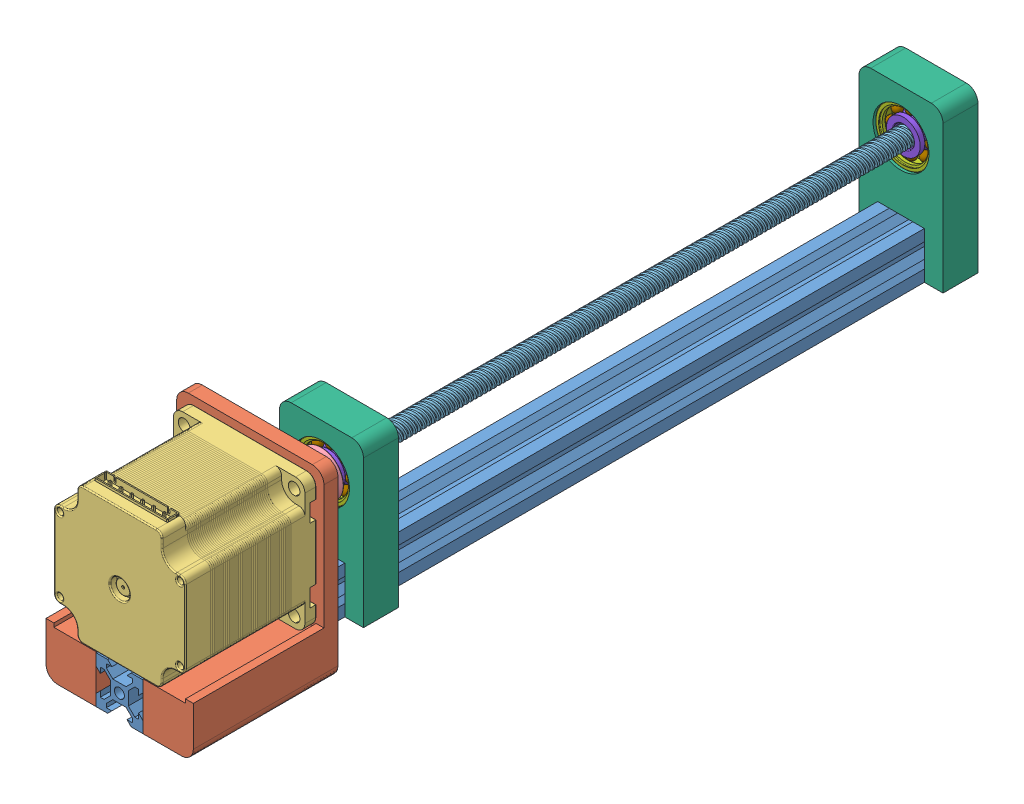
SolidWorks assembly AxisX, configuration Predeterminado. Lengths in mm.
Overall size (63.14 80.17 353.48).
17 component instances, 9 part files, 16 mates.
Components (placement in the parent):
- BoschAxisX-1: BoschAxisX [Predeterminado] at (-15.1935 9.652 175) size (20 20 350)
- NEMA-SupportX-1: NEMA-SupportX [Predeterminado] at (-28.6635 61.822 463) size (63.14 80.17 62)
- Nema 23-2: Nema 23 [Default] at (-5.0935 38.252 525) x (-1 0 0) z (0 0 -1) size (56.4 59.4 76.6)
- Coupler 6.35-8mm-1: Coupler 6.35-8mm [Default] at (-5.0935 38.252 450.9) x (0.753134 0.657867 0) z (0 0 1) size (19.34 19.34 25)
- ScrewAxisX-1: ScrewAxisX [Default] at (-5.0935 38.252 573.4) x (0.923728 0.383049 0) z (0 0 1) size (8.33 8.33 279.26)
- SupportX-1: SupportX [Predeterminado] at (16.5604 19.465 362.9) size (36 68 15)
  - SupportX-1: SupportX [Predeterminado] at (-31.754 -9.813 60.5) size (36 68 15)
  - skf_bearing_609_2-1: skf_bearing_609_2 [Default] at (-21.754 18.787 74.5) x (0 0 -1) z (1 0 0) size (7 24 24)
    - skf_bearing_609_2_01-1: skf_bearing_609_2_01 [Default] at origin size (7 24 24)
    - skf_bearing_609_2_02-1: skf_bearing_609_2_02 [Default] at origin size (7 14.45 14.45)
    - skf_bearing_609_2_03-1: skf_bearing_609_2_03 [Default] at origin size (3.97 20.97 20.97)
- SupportX-2: SupportX [Predeterminado] at (16.5604 19.465 114.5) size (36 68 15)
  - SupportX-1: SupportX [Predeterminado] at (-31.754 -9.813 60.5) size (36 68 15)
  - skf_bearing_609_2-1: skf_bearing_609_2 [Default] at (-21.754 18.787 74.5) x (0 0 -1) z (1 0 0) size (7 24 24)
    - skf_bearing_609_2_01-1: skf_bearing_609_2_01 [Default] at origin size (7 24 24)
    - skf_bearing_609_2_02-1: skf_bearing_609_2_02 [Default] at origin size (7 14.45 14.45)
    - skf_bearing_609_2_03-1: skf_bearing_609_2_03 [Default] at origin size (3.97 20.97 20.97)
Mates (geometry in assembly coordinates):
- Coincidente1: coincident aligned: plane of BoschAxisX-1 through (-15.1935 9.652 525) normal (0 0 1); plane of NEMA-Support-1 through (-28.6635 61.822 525) normal (0 0 1)
- Coincidente2: coincident anti-aligned: plane of BoschAxisX-1 through (-15.1935 9.652 525) normal (-1 0 0); plane of NEMA-Support-1 through (-15.1935 61.822 463) normal (1 0 0)
- Coincidente3: coincident aligned: plane of BoschAxisX-1 through (-15.1935 -10.348 525) normal (0 -1 0); plane of NEMA-Support-1 through (-28.6635 -10.348 463) normal (0 -1 0)
- Coincidente4: coincident anti-aligned: plane of NEMA-Support-1 through (-28.6635 61.822 469) normal (0 0 1); plane of Nema 23-2 through (19.1065 14.052 469) normal (0 0 -1)
- Concéntrica1: concentric anti-aligned: cylinder of NEMA-Support-1 through (-5.0935 38.252 469) axis (0 0 -1) radius 20; cylinder of Nema 23-2 through (-5.0935 38.252 467.4) axis (0 0 1) radius 19.05
- Paralelo1: parallel aligned: plane of NEMA-Support-1 through (26.4765 61.822 469) normal (1 0 0); plane of Nema 23-2 through (23.1065 53.952 514.2) normal (1 0 0)
- Concéntrica2: concentric aligned: cylinder of Nema 23-2 through (-5.0935 38.252 463.4) axis (0 0 1) radius 3.175; cylinder of Coupler 6.35-8mm-1 through (-5.0935 38.252 453.4) axis (0 0 1) radius 3.175
- Coincidente5: coincident anti-aligned: plane of Nema 23-2 through (-5.0935 38.252 463.4) normal (0 0 -1); plane of Coupler 6.35-8mm-1 through (-5.0935 38.252 463.4) normal (0 0 1)
- Coincidente6: coincident anti-aligned: plane of Nema 23-2 through (-5.0935 38.252 448.4) normal (0 0 -1); plane of ScrewAxisX-1 through (-5.0935 38.252 448.4) normal (0 0 1)
- Concéntrica3: concentric anti-aligned: circle of Coupler 6.35-8mm-1; circle of ScrewAxisX-1
- Coincidente7: coincident anti-aligned: plane of BoschAxisX-1 through (4.8065 9.652 525) normal (1 0 0); plane of ScrewSupport&Bearing-1/ScrewSupport-1 through (4.8065 9.652 438.4) normal (-1 0 0)
- Coincidente8: coincident aligned: plane of BoschAxisX-1 through (-15.1935 -10.348 525) normal (0 -1 0); plane of ScrewSupport&Bearing-1/ScrewSupport-1 through (-15.1935 -10.348 438.4) normal (0 -1 0)
- Coincidente9: coincident anti-aligned: plane of Coupler 6.35-8mm-1 through (-5.0935 38.252 438.4) normal (0 0 -1); plane of ScrewSupport&Bearing-1/ScrewSupport-1 through (-15.1935 9.652 438.4) normal (0 0 1)
- Coincidente10: coincident aligned: plane of BoschAxisX-1 through (-15.1935 9.652 175) normal (0 0 -1); plane of ScrewSupport&Bearing-2/ScrewSupport-1 through (-15.1935 9.652 175) normal (0 0 -1)
- Coincidente11: coincident anti-aligned: plane of BoschAxisX-1 through (4.8065 9.652 525) normal (1 0 0); plane of ScrewSupport&Bearing-2/ScrewSupport-1 through (4.8065 9.652 190) normal (-1 0 0)
- Coincidente12: coincident aligned: plane of BoschAxisX-1 through (-15.1935 -10.348 525) normal (0 -1 0); plane of ScrewSupport&Bearing-2/ScrewSupport-1 through (-15.1935 -10.348 190) normal (0 -1 0)
